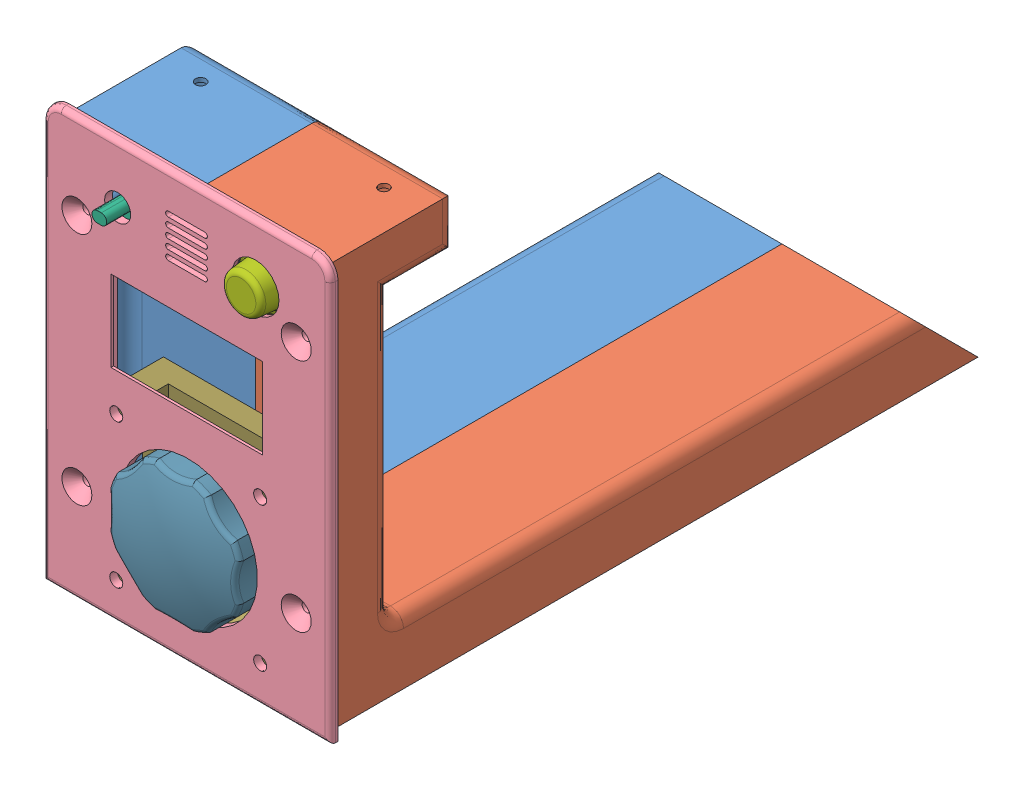
SolidWorks assembly Assy_box_control, configuration Default. Lengths in mm.
Overall size (110 187.12 285.79).
19 component instances, 15 part files, 28 mates.
Components (placement in the parent):
- box-control_D-1: box-control_D [Default] at (-180.6357 49.0448 463.5359) size (50.1 155 250)
- box-control_I-1: box-control_I [Default] at (-82.0357 49.0448 463.5359) size (50.1 155 250)
- base_control_box-1: base_control_box [Default] at (-178.5357 49.0448 465.1037) size (96 25 220)
- frente_control_box-1: frente_control_box [Default] at (-185.5357 49.0448 463.5359) size (110 160 8.5)
- DS3231 RTC-2: DS3231 RTC [Default] at (-98.9357 55.5448 310.9359) x (0 0 -1) z (0 -1 0) size (44.75 22.8 13.53)
  - Default-1: Default [Predeterminado] at origin size (44.75 22.8 13.53)
- LDR-1: LDR [Default] at (-156.876 173.9735 458.6019) x (1 0 0) z (0 0 -1) size (14.2 40.8 21.6)
- MQ135_sensor-1: MQ135_sensor [Default] at (-98.6357 185.4448 458.0359) x (0 1 0) z (0 0 1) size (36.7 20 20.1)
- ESP32_breadboard-1: ESP32_breadboard [Predeterminado] at (-142.2857 27.4234 204.8986) x (0 0 -1) z (1 0 0) size (186.74 40.42 55.48)
  - placa breadboard-1: placa breadboard [Predeterminado] at (-172.7373 28.1214 24.25) size (136 1.8 48.5)
  - 20-Pin Header - Female - 2.54mm-1: 20-Pin Header - Female - 2.54mm [Predeterminado] at (-93.0773 29.9214 11.43) size (51.3 8 2.5)
  - 20-Pin Header - Female - 2.54mm-2: 20-Pin Header - Female - 2.54mm [Predeterminado] at (-93.0773 29.9214 -11.43) size (51.3 8 2.5)
  - PCB_ESP32-38Pines-1: PCB_ESP32-38Pines [Predeterminado] at (-67.3173 36.9214 0) x (0 0 -1) z (1 0 0) size (28 10.12 55.48)
- perilla-1: perilla [Predeterminado] at (-127.2204 86.8536 424.0509) size (65 65 36.44)
  - Rotary Encoder - KY-040-1: Rotary Encoder - KY-040 [Default] at (-4.2339 1.2762 17.985) size (19 30.75 32.39)
  - chasis_perilla-1: chasis_perilla [Predeterminado] at (-2.6839 3.7912 27.485) size (65 65 20.5)
  - rodamiento-1: rodamiento [Predeterminado] at (-2.6839 3.7912 33.485) x (1 0 0) z (0 -1 0) size (44.2 9 44.2)
  - perilla52-1: perilla52 [Predeterminado] at (-2.6839 3.7912 47.635) x (1 0 0) z (0 0 -1) size (52.46 52.46 20)
- LoRa_Module_RA-02-1: LoRa_Module_RA-02 [Predeterminado] at (-94.5357 55.5448 278.6359) x (1 0 0) z (0 1 0) size (16 17 3.03)
Mates (geometry in assembly coordinates):
- Coincident1: coincident aligned: plane of box-control_D-1 through (-179.0357 74.0448 238.5359) normal (0 1 0); plane of box-control_I-1 through (-80.4357 74.0448 238.5359) normal (0 1 0)
- Coincident2: coincident aligned: plane of box-control_D-1 through (-130.5357 74.0448 238.5359) normal (0 0 -1); plane of box-control_I-1 through (-130.5357 74.0448 238.5359) normal (0 0 -1)
- Coincident3: coincident anti-aligned: plane of box-control_D-1 through (-130.5357 49.0448 463.5359) normal (1 0 0); plane of box-control_I-1 through (-130.5357 49.0448 463.5359) normal (-1 0 0)
- Concentric1: concentric aligned: cylinder of box-control_D-1 through (-172.0357 204.0468 250.1359) axis (0 -1 0) radius 1.5; cylinder of base_control_box-1 through (-172.0357 54.0448 250.1359) axis (0 -1 0) radius 3
- Concentric2: concentric aligned: cylinder of box-control_D-1 through (-172.0357 204.0468 430.1359) axis (0 -1 0) radius 1.5; cylinder of base_control_box-1 through (-172.0357 54.0448 430.1359) axis (0 -1 0) radius 3
- Coincident4: coincident anti-aligned: plane of box-control_D-1 through (-177.3976 55.0448 254.6359) normal (0 -1 0); plane of base_control_box-1 through (-385.4101 55.0448 239.6359) normal (0 1 0)
- Coincident5: coincident anti-aligned: plane of box-control_D-1 through (-179.0357 204.0448 463.5359) normal (0 0 1); plane of frente_control_box-1 through (-178.5357 202.0448 463.5359) normal (0 0 -1)
- Width1: width anti-aligned: plane of box-control_D-1 through (-180.6357 49.0448 463.5359) normal (-1 0 0); plane of frente_control_box-1 through (-80.4357 49.0448 463.5359) normal (1 0 0); plane of box-control_I-1 through (-75.5357 49.0448 466.5359) normal (1 0 0); plane of frente_control_box-1 through (-185.5357 49.0448 466.5359) normal (-1 0 0)
- Coincident6: coincident aligned: plane of box-control_I-1 through (-80.4357 49.0448 463.5359) normal (0 -1 0); plane of frente_control_box-1 through (-185.5357 49.0448 466.5359) normal (0 -1 0)
- Distance3: distance = 5 mm: plane of DS3231 RTC-2/Default-1 through (-98.9357 55.5448 310.9359) normal (0 -1 0); plane of base_control_box-1 through (-89.0357 50.5448 250.1359) normal (0 1 0)
- Distance4: distance = 50 mm anti-aligned: plane of base_control_box-1 through (-84.5357 50.5448 241.6359) normal (0 0 1); plane of DS3231 RTC-2/Default-1 through (-87.5357 57.1448 291.6359) normal (0 0 -1)
- Distance5: distance = 3 mm anti-aligned: plane of base_control_box-1 through (-84.5357 50.5448 425.6359) normal (-1 0 0); plane of DS3231 RTC-2/Default-1 through (-87.5357 57.1448 330.2359) normal (1 0 0)
- Distance9: coincident anti-aligned: plane of frente_control_box-1 through (-156.9357 165.1948 458.5359) normal (0 0 -1); plane of LDR-1 through (-156.876 173.9735 458.5359) normal (0 0 1)
- Distance12: distance = 5.5 mm anti-aligned: plane of MQ135_sensor-1 through (-104.1357 182.9448 458.0359) normal (0 0 1); plane of frente_control_box-1 through (-178.5357 202.0448 463.5359) normal (0 0 -1)
- Distance15: distance = 1 mm anti-aligned: plane of MQ135_sensor-1 through (-114.1357 198.9448 458.0359) normal (0 1 0); plane of frente_control_box-1 through (-84.1357 199.9448 459.6359) normal (0 -1 0)
- Distance16: distance = 10 mm anti-aligned: plane of MQ135_sensor-1 through (-94.1357 198.9448 458.0359) normal (1 0 0); plane of frente_control_box-1 through (-84.1357 180.5448 459.6359) normal (-1 0 0)
- Distance17: parallel anti-aligned: plane of frente_control_box-1 through (-84.1357 199.9448 459.6359) normal (0 -1 0); plane of LDR-1 through (-164.0357 189.6948 458.5359) normal (0 1 0)
- Width2: width: plane of LDR-1 through (-156.1857 189.0248 473.5359) normal (0 1 0); plane of frente_control_box-1 through (-156.1857 184.8648 473.5359) normal (0 -1 0); cylinder of LDR-1 through (-156.9357 186.9448 466.5359) axis (0 0 -1) radius 5
- Distancia4: distance = 5 mm anti-aligned: plane of base_control_box-1 through (-89.0357 50.5448 250.1359) normal (0 1 0); plane of ESP32_breadboard-1/placa breadboard-1 through (-118.0357 55.5448 377.6359) normal (0 -1 0)
- Coincidente8: coincident anti-aligned: plane of base_control_box-1 through (-84.5357 50.5448 241.6359) normal (0 0 1); plane of ESP32_breadboard-1/placa breadboard-1 through (-118.0357 57.3448 241.6359) normal (0 0 -1)
- Distancia6: distance = 10 mm anti-aligned: plane of ESP32_breadboard-1/placa breadboard-1 through (-166.5357 57.3448 377.6359) normal (-1 0 0); plane of base_control_box-1 through (-176.5357 50.5448 254.6359) normal (1 0 0)
- Ancho1: width: plane of LDR-1 through (-149.8357 189.6948 458.5359) normal (1 0 0); plane of LDR-1 through (-164.0357 158.1948 458.5359) normal (-1 0 0); cylinder of frente_control_box-1 through (-156.9357 186.9448 466.5359) axis (0 0 -1) radius 5
- Coincidente7: coincident anti-aligned: plane of frente_control_box-1 through (-178.5357 202.0448 463.5359) normal (0 0 -1); plane of perilla-1/chasis_perilla-1 through (-157.5047 118.2453 463.5359) normal (0 0 1)
- Concéntrica1: concentric anti-aligned: cylinder of frente_control_box-1 through (-157.4545 118.1951 466.5369) axis (0 0 -1) radius 2.5; cylinder of perilla-1/chasis_perilla-1 through (-157.4545 118.1951 443.5359) axis (0 0 1) radius 2.5
- Concéntrica2: concentric anti-aligned: cylinder of frente_control_box-1 through (-102.354 118.1951 466.5369) axis (0 0 -1) radius 2.5; cylinder of perilla-1/chasis_perilla-1 through (-102.354 118.1951 443.5359) axis (0 0 1) radius 2.5
- Distancia7: distance = 5 mm anti-aligned: plane of base_control_box-1 through (-89.0357 50.5448 250.1359) normal (0 1 0); plane of LoRa_Module_RA-02-1 through (-102.5357 55.5448 270.1359) normal (0 -1 0)
- Distancia8: distance = 10 mm anti-aligned: plane of LoRa_Module_RA-02-1 through (-94.5357 56.7948 267.5859) normal (1 0 0); plane of base_control_box-1 through (-84.5357 50.5448 425.6359) normal (-1 0 0)
- Distancia9: distance = 20 mm anti-aligned: plane of base_control_box-1 through (-84.5357 50.5448 241.6359) normal (0 0 1); plane of LoRa_Module_RA-02-1 through (-102.5357 56.1698 261.6359) normal (0 0 -1)
